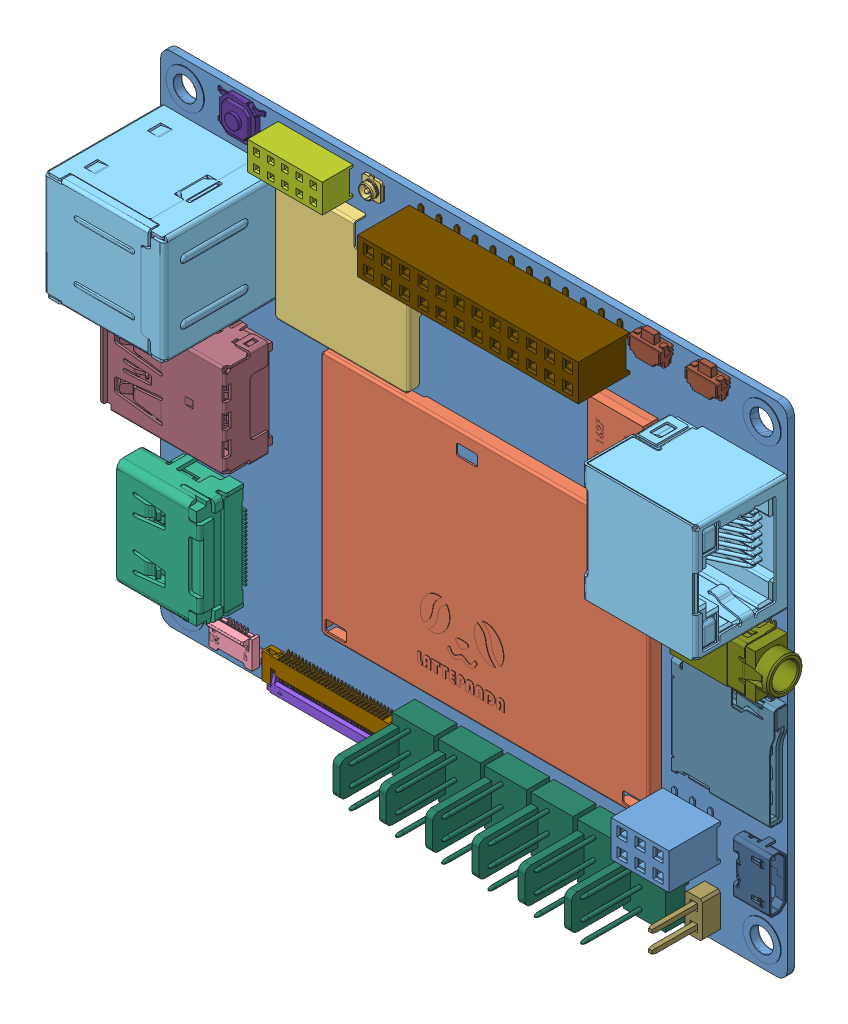
SolidWorks assembly LattePanda v0.1 3D Model, configuration Default. Lengths in mm.
Overall size (90.8 70.68 21.36).
30 component instances, 23 part files, 7 mates.
Components (placement in the parent):
- PCB-1: PCB [Default] at origin size (88 70 1.2)
- S70CR100_LED_SKT-1: S70CR100_LED_SKT [Default] at (-0.725 -6.25 1) size (46.05 34.5 1.85)
- S70CR100_RF_SKT-1: S70CR100_RF_SKT [Default] at (0 0 1) size (18.9 17.35 1.81)
- S70CR100_SOC_SKT-1: S70CR100_SOC_SKT [Default] at origin size (46.3 50.4 1.8)
- ASM0001_ASM_22_AF0_ASM-2: ASM0001_ASM_22_AF0_ASM [Default] at (24.55 18.525 7.3) x (0 1 0) z (1 0 0) size (16.45 17.03 15.85)
- hdmi-krps00-a30n2-l_asm_6-1: hdmi-krps00-a30n2-l_asm_6 [Default] at (-49.05 -20 4.4054) x (0 1 0) z (1 0 0) size (15.01 8.36 12.11)
- STP_62001021821-1: STP_62001021821 [Default] at (-26.25 32 3.15) size (10.5 4 6.7)
- FPC0515_30PIN-2: FPC0515_30PIN [Default] at (-32.3 -34.5 0.965) x (0 1 0) z (0 0 -1) size (5 19.1 1.54)
  - FPC0515_30PIN - Keylock-1: FPC0515_30PIN - Keylock [Default] at origin size (2.34 17.7 1.3)
  - FPC0515_30PIN Body part-1: FPC0515_30PIN Body part [Default] at origin size (4.2 19.1 1.54)
- 4_85MM_3D-1: 4_85MM_3D [Default] at (40 -22.25 3.2) x (0 1 0) z (1 0 0) size (7.5 3.6 5.37)
- ASM0015_ASM_1_ASM_1_ASM_ASM_ASM-3: ASM0015_ASM_1_ASM_1_ASM_ASM_ASM [Default] at (29.725 33.98 2.82) x (-1 0 0) z (0 0 -1) size (4.55 3.48 2.4)
- ASM0015_ASM_1_ASM_1_ASM_ASM_ASM-4: ASM0015_ASM_1_ASM_1_ASM_ASM_ASM [Default] at (21.725 33.98 2.82) x (-1 0 0) z (0 0 -1) size (4.55 3.48 2.4)
- PZ_254_2P ASM-1: PZ_254_2P ASM [Default] at (29.35 -30.96 1) x (0 1 0) z (0 0 1) size (5.08 2.5 11.6)
- USB3_0-001-ANBL_2_0_-LH REBUILD-1: USB3_0-001-ANBL_2_0_-LH REBUILD [Default] at (-35.92 0.55 5.11) x (0 -1 0) z (-1 0 0) size (15.8 11.53 17)
- PRT0112 ASM Rebuild-1: PRT0112 ASM Rebuild [Default] at (32.75 -8.38 2.65) x (0 1 0) z (0 0 1) size (16.15 15.1 2.41)
- PAIZHEN Rebuild-1: PAIZHEN Rebuild [Default] at (-38.3 -5.25 -0.6) size (5.9 7.6 14.51)
- PAIZHEN Rebuild-2: PAIZHEN Rebuild [Default] at (-31.8 -5.25 -0.6) size (5.9 7.6 14.51)
- PAIZHEN Rebuild-3: PAIZHEN Rebuild [Default] at (-25.3 -5.25 -0.6) size (5.9 7.6 14.51)
- PAIZHEN Rebuild-4: PAIZHEN Rebuild [Default] at (-18.8 -5.25 -0.6) size (5.9 7.6 14.51)
- PAIZHEN Rebuild-5: PAIZHEN Rebuild [Default] at (-12.3 -5.25 -0.6) size (5.9 7.6 14.51)
- PAIZHEN Rebuild-6: PAIZHEN Rebuild [Default] at (-5.8 -5.25 -0.6) size (5.9 7.6 14.51)
- _J305B06G13ZL2 Rebuild ASM Not accurate-1: _J305B06G13ZL2 Rebuild ASM Not accurate [Default] at (34.4 4.415 5.5) size (14 7.55 5.4)
- microswitch-1: microswitch [Default] at (-36.508 32.1916 1) x (1 0 0) z (0 -1 0) size (6.55 1.56 5.05)
- STP_61002421821-1: STP_61002421821 [Default] at (2.6047 30.6931 4.83) size (30.98 6.7 7.45)
- STP_61002421821Rebuild 3pin-1: STP_61002421821Rebuild 3pin [Default] at (38.1944 -22.3679 4.83) size (8.14 6.7 7.45)
- pfs 1-1: pfs 1 [Default] at (19.6704 18.2622 1) x (-1 0 0) z (0 0 1) size (10.5 12.81 2.14)
- kfm110z-1002-7f-1: kfm110z-1002-7f [Default] at (-18.0506 32.7317 2.25) x (0 0 -1) z (1 0 0) size (1.29 3.1 3)
- FPC 6pin Rebuild unaccurate pins-1: FPC 6pin Rebuild unaccurate pins [Default] at (-36.97 -1032.2241 -1599.9866) x (0 1 0) z (1 0 0) size (3.8 2.27 7.19)
- USB2.0_2_sheild-1: USB2.0_2_sheild [Default] at (-39.55 28.15 17.45) x (1 0 0) z (0 -1 0) size (17.15 21.36 15.6)
Mates (geometry in assembly coordinates):
- Coincident4: coincident anti-aligned: plane of PCB-1 through (0 0 1) normal (0 0 1); plane of STP_62001021821-1 through (-21 30 1) normal (0 0 -1)
- Coincident5: coincident anti-aligned: plane of PCB-1 through (0 0 1) normal (0 0 1); plane of FPC0515_30PIN-2/FPC0515_30PIN Body part-1 through (-30.7775 -31.925 1) normal (0 0 -1)
- Coincident6: coincident anti-aligned: plane of PCB-1 through (0 0 1) normal (0 0 1); plane of microswitch-1 through (-36.508 32.1916 1) normal (0 0 -1)
- Coincident9: coincident anti-aligned: plane of PCB-1 through (0 0 1) normal (0 0 1); plane of STP_61002421821-1 through (-11.0453 32.9231 1) normal (0 0 -1)
- Coincident10: coincident anti-aligned: plane of PCB-1 through (0 0 1) normal (0 0 1); plane of STP_61002421821Rebuild 3pin-1 through (24.5444 -20.1379 1) normal (0 0 -1)
- Coincident11: coincident anti-aligned: plane of PCB-1 through (0 0 1) normal (0 0 1); plane of pfs 1-1 through (13.8752 18.4168 1) normal (0 0 -1)
- Coincident12: coincident anti-aligned: plane of PCB-1 through (0 0 1) normal (0 0 1); plane of kfm110z-1002-7f-1 through (-19.4026 34.0837 1) normal (0 0 -1)
